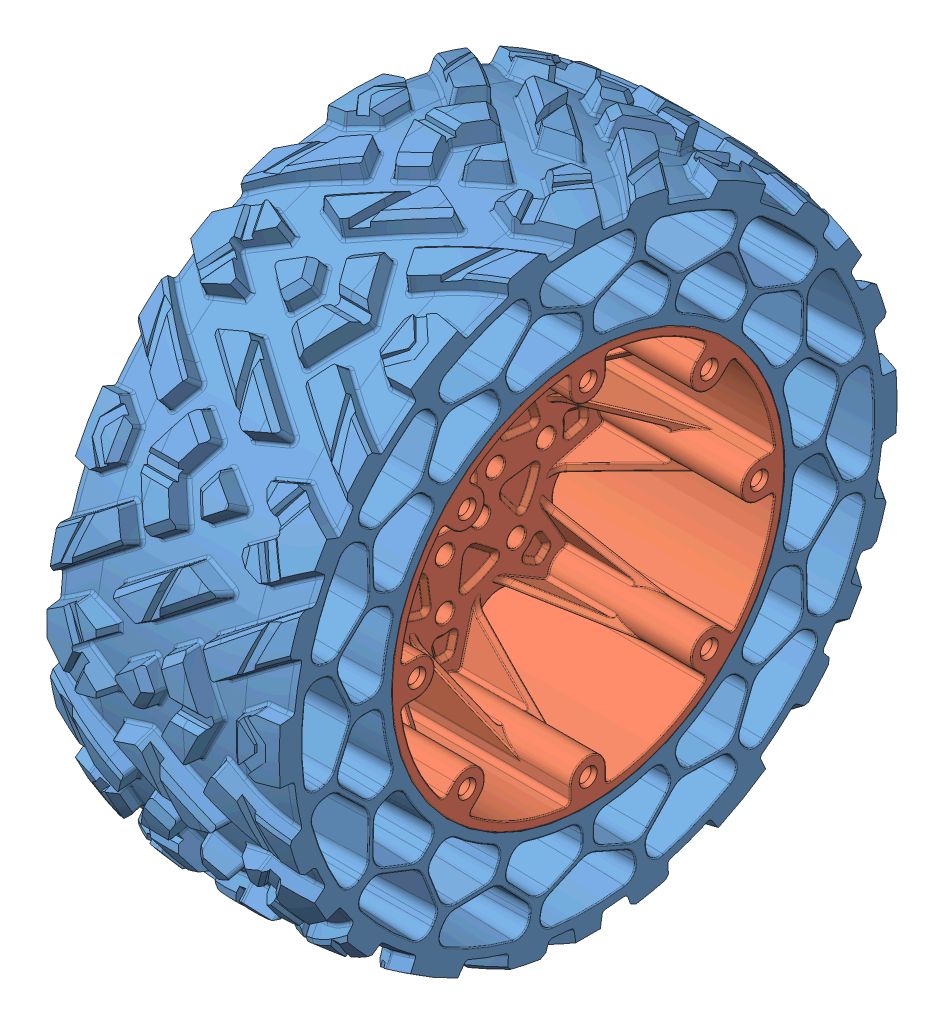
SolidWorks assembly 3616-0014-0144 Assembly, configuration Défaut. Lengths in mm.
Overall size (53.03 144.24 144.24).
3 component instances, 2 part files, 0 mates.
Components (placement in the parent):
- 3616-0014-0144 Assembly.step-1: 3616-0014-0144 Assembly.step [Défaut] at origin size (53.03 144.24 144.24)
  - Rubber V0.5 88mm.step-1: Rubber V0.5 88mm.step [Défaut] at (34 0 0) x (0 0 -1) z (1 0 0) size (144.24 144.24 53.03)
  - Rim 88mm V13.step-1: Rim 88mm V13.step [Défaut] at origin size (52.06 90.7 90.7)
